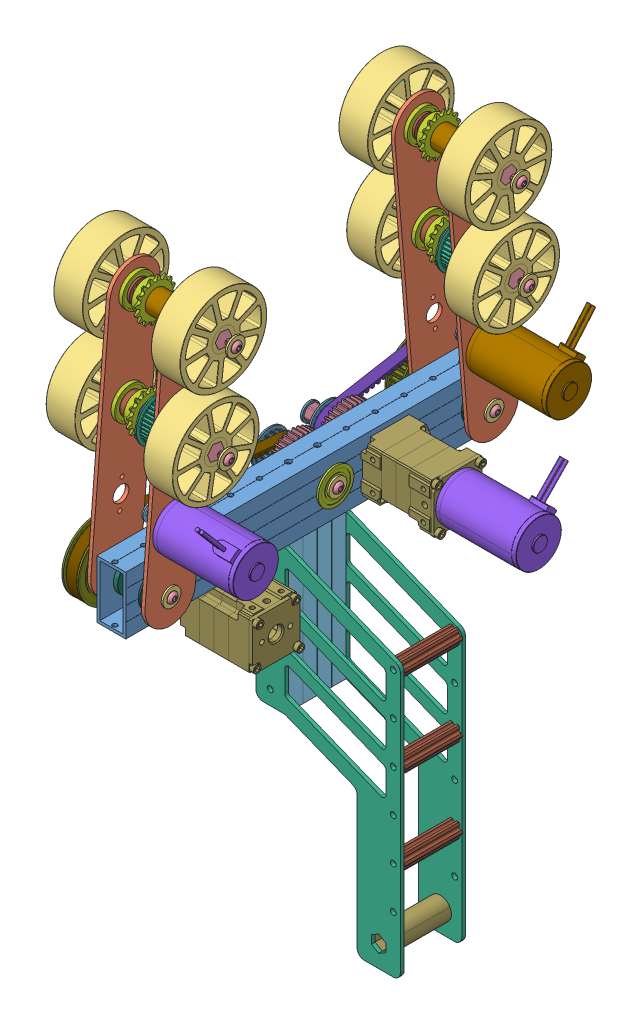
SolidWorks assembly updated grabber, configuration Default. Lengths in mm.
Overall size (217.61 560.62 367.28).
125 component instances, 32 part files, 6 mates.
Components (placement in the parent):
- 18000 - Rotational Grabber-1: 18000 - Rotational Grabber [Default] at (150.3363 402.3193 -558.2646) size (217.61 560.62 367.28)
  - 18001 - 11in Base Versaframe-1: 18001 - 11in Base Versaframe [Default] at (-59.9903 -66.9277 445.6815) size (25.4 50.8 336.55)
  - 18002 - Grabber intake plate-1: 18002 - Grabber intake plate [Default] at (-85.3649 -68.7494 1136.9284) x (0 0.081964 0.996635) z (0 0.996635 -0.081964) size (44.45 3.17 247.65)
  - 18002 - Grabber intake plate-2: 18002 - Grabber intake plate [Default] at (-85.3649 -65.1061 853.1342) x (0 -0.081964 0.996635) z (0 0.996635 0.081964) size (44.45 3.17 247.65)
  - 18002 - Grabber intake plate-3: 18002 - Grabber intake plate [Default] at (-34.6157 -68.7494 897.4346) x (0 0.081964 -0.996635) z (0 0.996635 0.081964) size (44.45 3.17 247.65)
  - 18002 - Grabber intake plate-4: 18002 - Grabber intake plate [Default] at (-34.6157 -65.1061 1181.2288) x (0 -0.081964 -0.996635) z (0 0.996635 -0.081964) size (44.45 3.17 247.65)
  - Andymark - 3in .5in Hex Compliant Wheel am-3945-1: Andymark - 3in .5in Hex Compliant Wheel am-3945 [Default] at (11.4119 85.6619 1174.5787) x (0 -0.802579 0.596545) z (-1 0 0) size (76.2 76.2 25.4)
  - Andymark - 3in .5in Hex Compliant Wheel am-3945-2: Andymark - 3in .5in Hex Compliant Wheel am-3945 [Default] at (11.4119 180.7711 930.4775) x (0 0.802579 0.596545) z (-1 0 0) size (76.2 76.2 25.4)
  - Andymark - 3in .5in Hex Compliant Wheel am-3945-3: Andymark - 3in .5in Hex Compliant Wheel am-3945 [Default] at (-74.2623 85.6619 1174.5787) x (0 -0.802579 0.596545) z (-1 0 0) size (76.2 76.2 25.4)
  - Andymark - 3in .5in Hex Compliant Wheel am-3945-4: Andymark - 3in .5in Hex Compliant Wheel am-3945 [Default] at (-131.3925 185.5152 924.0948) x (0 0.802579 0.596545) z (1 0 0) size (76.2 76.2 25.4)
  - Andymark - 3in .5in Hex Compliant Wheel am-3945-5: Andymark - 3in .5in Hex Compliant Wheel am-3945 [Default] at (-45.7183 67.5471 1206.8448) x (0 0.174088 0.98473) z (1 0 0) size (76.2 76.2 25.4)
  - Andymark - 3in .5in Hex Compliant Wheel am-3945-6: Andymark - 3in .5in Hex Compliant Wheel am-3945 [Default] at (-45.7183 59.7158 826.1337) x (0 0.174088 -0.98473) z (1 0 0) size (76.2 76.2 25.4)
  - Andymark - 3in .5in Hex Compliant Wheel am-3945-7: Andymark - 3in .5in Hex Compliant Wheel am-3945 [Default] at (-74.2623 46.9169 1090.1499) x (0 -0.174088 -0.98473) z (-1 0 0) size (76.2 76.2 25.4)
  - Andymark - 3in .5in Hex Compliant Wheel am-3945-8: Andymark - 3in .5in Hex Compliant Wheel am-3945 [Default] at (-74.2623 39.0856 942.8286) x (0 -0.174088 0.98473) z (-1 0 0) size (76.2 76.2 25.4)
  - 18003 -  Intake Shaft 4.75 in-4: 18003 -  Intake Shaft 4.75 in [Default] at (-461.6532 135.6003 1142.4147) x (0 -0.802579 0.596545) z (-1 0 0) size (14.48 12.67 120.65)
  - 18003 -  Intake Shaft 4.75 in-5: 18003 -  Intake Shaft 4.75 in [Default] at (-461.6532 53.2963 1149.2065) x (0 0.765757 -0.64313) z (-1 0 0) size (14.48 12.67 120.65)
  - 17001 - Intake Mounting Versaframe-1: 17001 - Intake Mounting Versaframe [Default] at (-59.9903 -841.6277 1017.1815) x (1 0 0) z (0 -1 0) size (25.4 50.8 127)
  - 17003 - Intake Mounting Platwe-1: 17003 - Intake Mounting Platwe [Default] at (-72.6903 -92.3277 1042.5815) x (0 -1 0) z (0 0 1) size (279.4 127 3.17)
  - 17003 - Intake Mounting Platwe-2: 17003 - Intake Mounting Platwe [Default] at (-72.6903 -92.3277 988.6065) x (0 -1 0) z (0 0 1) size (279.4 127 3.17)
  - Vexpro - .5in hex bearing flanged - 217-3875-13: Vexpro - .5in hex bearing flanged - 217-3875 [Default] at (-40.9657 53.3163 1149.1896) x (0 -0.765757 0.64313) z (0 0.64313 0.765757) size (31.12 7.94 31.12)
  - Vexpro - .5in hex bearing flanged - 217-3875-15: Vexpro - .5in hex bearing flanged - 217-3875 [Default] at (-40.9657 135.5886 1142.4234) x (0 0.917913 0.396782) z (0 0.396782 -0.917913) size (31.12 7.94 31.12)
  - Vexpro - .5in hex bearing flanged - 217-3875-16: Vexpro - .5in hex bearing flanged - 217-3875 [Default] at (-40.9657 53.3163 885.1734) x (0 -0.950153 0.311785) z (0 0.311785 0.950153) size (31.12 7.94 31.12)
  - Vexpro - .5in hex bearing flanged - 217-3875-17: Vexpro - .5in hex bearing flanged - 217-3875 [Default] at (-40.9657 135.5886 891.9395) x (0 -0.202349 0.979313) z (0 0.979313 0.202349) size (31.12 7.94 31.12)
  - Vexpro - .5in hex bearing flanged - 217-3875-19: Vexpro - .5in hex bearing flanged - 217-3875 [Default] at (-79.0149 135.5886 1142.4234) x (0 0.917913 0.396782) z (0 -0.396782 0.917913) size (31.12 7.94 31.12)
  - Vexpro - .5in hex bearing flanged - 217-3875-20: Vexpro - .5in hex bearing flanged - 217-3875 [Default] at (-79.0149 53.3163 1149.1896) x (0 -0.765757 0.64313) z (0 -0.64313 -0.765757) size (31.12 7.94 31.12)
  - Vexpro - .5in hex bearing flanged - 217-3875-21: Vexpro - .5in hex bearing flanged - 217-3875 [Default] at (-79.0149 135.5886 891.9395) x (0 -0.202349 0.979313) z (0 -0.979313 -0.202349) size (31.12 7.94 31.12)
  - Vexpro - .5in hex bearing flanged - 217-3875-22: Vexpro - .5in hex bearing flanged - 217-3875 [Default] at (-79.0149 53.3163 885.1734) x (0 -0.950153 0.311785) z (0 -0.311785 -0.950153) size (31.12 7.94 31.12)
  - Vexpro - BAG Motor - 217-3351-2: Vexpro - BAG Motor - 217-3351 [Default] at (-34.6157 -14.5013 1154.767) x (0 -0.996635 0.081964) z (-1 0 0) size (59.07 59.07 84.5)
  - 18003 -  Intake Shaft 4.75 in-6: 18003 -  Intake Shaft 4.75 in [Default] at (332.0968 53.2963 885.1565) x (0 0.765757 0.64313) z (1 0 0) size (14.48 12.67 120.65)
  - 18003 -  Intake Shaft 4.75 in-7: 18003 -  Intake Shaft 4.75 in [Default] at (332.0968 135.6003 891.9483) x (0 -0.802579 -0.596545) z (1 0 0) size (14.48 12.67 120.65)
  - MirrorVexpro - BAG Motor - 217-3351-3: MirrorVexpro - BAG Motor - 217-3351 [Default] at (-34.6157 -14.5013 879.596) x (0 -0.996635 -0.081964) z (1 0 0) size (59.07 59.07 84.5)
  - Vexpro - .125 acetal hex spacer - 217-2758-1: Vexpro - .125 acetal hex spacer - 217-2758 [Default] at (-31.4407 135.5886 891.9395) x (0 0.919668 0.392697) z (-1 0 0) size (19.05 19.05 3.17)
  - Vexpro - .125 acetal hex spacer - 217-2758-2: Vexpro - .125 acetal hex spacer - 217-2758 [Default] at (-31.4407 135.5886 1142.4234) x (0 0.919668 -0.392697) z (1 0 0) size (19.05 19.05 3.17)
  - Vexpro - .125 acetal hex spacer - 217-2758-3: Vexpro - .125 acetal hex spacer - 217-2758 [Default] at (-31.4407 53.3163 885.1734) x (0 0.919668 0.392697) z (-1 0 0) size (19.05 19.05 3.17)
  - Vexpro - .125 acetal hex spacer - 217-2758-4: Vexpro - .125 acetal hex spacer - 217-2758 [Default] at (-31.4407 53.3163 1149.1896) x (0 0.919668 -0.392697) z (1 0 0) size (19.05 19.05 3.17)
  - Vexpro - .125 acetal hex spacer - 217-2758-5: Vexpro - .125 acetal hex spacer - 217-2758 [Default] at (-88.5399 135.5886 891.9395) x (0 0.919668 0.392697) z (-1 0 0) size (19.05 19.05 3.17)
  - Vexpro - .125 acetal hex spacer - 217-2758-6: Vexpro - .125 acetal hex spacer - 217-2758 [Default] at (-88.5399 53.3163 885.1734) x (0 0.919668 0.392697) z (-1 0 0) size (19.05 19.05 3.17)
  - Vexpro - .125 acetal hex spacer - 217-2758-7: Vexpro - .125 acetal hex spacer - 217-2758 [Default] at (-88.5399 135.5886 1142.4234) x (0 0.919668 -0.392697) z (1 0 0) size (19.05 19.05 3.17)
  - Vexpro - .125 acetal hex spacer - 217-2758-8: Vexpro - .125 acetal hex spacer - 217-2758 [Default] at (-88.5399 53.3163 1149.1896) x (0 0.919668 -0.392697) z (1 0 0) size (19.05 19.05 3.17)
  - Vexpro - .25in acetal hex spacer - 217-3259-1: Vexpro - .25in acetal hex spacer - 217-3259 [Default] at (-75.8399 53.3163 885.1734) x (0 0.983572 0.180519) z (-1 0 0) size (19.5 19.5 6.35)
  - Vexpro - .25in acetal hex spacer - 217-3259-2: Vexpro - .25in acetal hex spacer - 217-3259 [Default] at (-75.8399 53.3163 1149.1896) x (0 0.983572 -0.180519) z (1 0 0) size (19.5 19.5 6.35)
  - Vexpro - .25in acetal hex spacer - 217-3259-5: Vexpro - .25in acetal hex spacer - 217-3259 [Default] at (-80.577 135.5886 891.9395) x (0 0.981987 0.188951) z (-1 0 0) size (19.5 19.5 6.35)
  - Vexpro - .25in acetal hex spacer - 217-3259-6: Vexpro - .25in acetal hex spacer - 217-3259 [Default] at (-80.577 135.5886 1142.4234) x (0 0.981987 -0.188951) z (1 0 0) size (19.5 19.5 6.35)
  - Vexpro - 100 to 1 BAG Versaplanetary Assembly-1: Vexpro - 100 to 1 BAG Versaplanetary Assembly [Default] at (-30.6653 -66.9277 934.2886) x (-1 0 0) z (0 1 0) size (107.67 44.45 42.65)
  - Vexpro - BAG Motor - 217-3351-3: Vexpro - BAG Motor - 217-3351 [Default] at (15.7347 -66.9277 956.5136) x (0 -0.014739 0.999891) z (-1 0 0) size (59.07 59.07 84.5)
  - Vexpro - 36t 20DP 0.5 Hex Gear, 217-3214-1: Vexpro - 36t 20DP 0.5 Hex Gear, 217-3214 [Default] at (-80.6024 -66.9277 956.5136) x (0 0.690037 0.723774) z (-1 0 0) size (48.16 48.16 12.65)
  - Vexpro - 36t 20DP 0.5 Hex Gear, 217-3214-2: Vexpro - 36t 20DP 0.5 Hex Gear, 217-3214 [Default] at (-80.6024 -66.9277 1002.2336) x (0 -0.981814 -0.189847) z (-1 0 0) size (48.16 48.16 12.65)
  - 18T x 9mm Wide Double Flange Aluminum Pulley (HTD 5mm, 1_2” Hex Bore) (217-3225)-1: 18T x 9mm Wide Double Flange Aluminum Pulley (HTD 5mm, 1_2” Hex Bore) (217-3225) [Default] at (-92.6149 -66.9277 956.5136) x (0 0.000638 -1) z (1 0 0) size (32 32 14.5)
  - 18T x 9mm Wide Double Flange Aluminum Pulley (HTD 5mm, 1_2” Hex Bore) (217-3225)-2: 18T x 9mm Wide Double Flange Aluminum Pulley (HTD 5mm, 1_2” Hex Bore) (217-3225) [Default] at (-97.352 -66.9277 1002.2336) x (0 0.755352 0.655319) z (-1 0 0) size (32 32 14.5)
  - Vexpro - .5in hex bearing flanged - 217-3875-27: Vexpro - .5in hex bearing flanged - 217-3875 [Default] at (-66.3403 -66.9277 956.5136) x (0 0.918835 -0.394642) z (0 0.394642 0.918835) size (31.12 7.94 31.12)
  - Vexpro - .5in hex bearing flanged - 217-3875-28: Vexpro - .5in hex bearing flanged - 217-3875 [Default] at (-66.3403 -66.9277 1002.2336) x (0 0.945199 -0.326495) z (0 0.326495 0.945199) size (31.12 7.94 31.12)
  - Vexpro - .5in hex bearing flanged - 217-3875-29: Vexpro - .5in hex bearing flanged - 217-3875 [Default] at (-53.6403 -66.9277 1002.2336) x (0 0.945199 -0.326495) z (0 -0.326495 -0.945199) size (31.12 7.94 31.12)
  - Vexpro - 13.75mm Thunderhex Bearing - 217-4006-1: Vexpro - 13.75mm Thunderhex Bearing - 217-4006 [Default] at (-49.6715 -66.9277 1159.0786) x (0 -0.259596 -0.965717) z (1 0 0) size (31.12 31.12 7.94)
  - Vexpro - 13.75mm Thunderhex Bearing - 217-4006-4: Vexpro - 13.75mm Thunderhex Bearing - 217-4006 [Default] at (-70.309 -66.9277 1159.0786) x (0 0.259596 0.965717) z (-1 0 0) size (31.12 31.12 7.94)
  - Vexpro - 13.75mm Thunderhex Bearing - 217-4006-3: Vexpro - 13.75mm Thunderhex Bearing - 217-4006 [Default] at (-49.6715 -66.9277 875.2844) x (0 0.259596 -0.965717) z (1 0 0) size (31.12 31.12 7.94)
  - Vexpro - 13.75mm Thunderhex Bearing - 217-4006-5: Vexpro - 13.75mm Thunderhex Bearing - 217-4006 [Default] at (-70.309 -66.9277 875.2844) x (0 -0.259596 0.965717) z (-1 0 0) size (31.12 31.12 7.94)
  - 36t Pulley HTD5-1: 36t Pulley HTD5 [Default] at (-92.6149 -66.9277 875.2844) x (0 -0.569301 0.822129) z (-1 0 0) size (60 60 14.5)
  - 60t Belt-2: 60t Belt [Default] at (-91.6149 -66.9277 915.899) x (0 0 -1) z (0 -1 0) size (126.54 9 59.64)
  - 90t Belt (1)-2: 90t Belt (1) [Default] at (-91.6149 -66.9277 1080.6561) x (0 0 1) z (0 1 0) size (202.16 9 59.64)
  - 36t Pulley HTD5-3: 36t Pulley HTD5 [Default] at (-92.6149 -66.9277 1159.0786) x (0 -0.569301 -0.822129) z (1 0 0) size (60 60 14.5)
  - 18004 - Intake Rotation Shaft-1: 18004 - Intake Rotation Shaft [Default] at (-491.8157 -66.6646 875.306) x (0 0.996635 0.081964) z (-1 0 0) size (13.74 12.75 74.93)
  - 18004 - Intake Rotation Shaft-2: 18004 - Intake Rotation Shaft [Default] at (347.6543 -66.6646 1159.057) x (0 0.996635 -0.081964) z (1 0 0) size (13.74 12.75 74.93)
  - Gear shaft 2-1: Gear shaft 2 [Default] at (-502.874 -66.9277 1002.2336) x (0 0.945199 -0.326495) z (-1 0 0) size (13.74 12.75 58.93)
  - McMaster - .25 ID washer - 96765A140-6: McMaster - .25 ID washer - 96765A140 [96765A140] at (-106.126 -66.9277 1002.2336) x (0 -0.992326 0.123647) z (0 0.123647 0.992326) size (15.88 1.52 15.88)
  - McMaster - .25 ID washer - 96765A140-7: McMaster - .25 ID washer - 96765A140 [96765A140] at (-45.7028 -66.9277 1002.2336) x (0 0.885672 -0.464312) z (0 -0.464312 -0.885672) size (15.88 1.52 15.88)
  - McMaster - 10-32 .3125in button head screw - 97763A706-7: McMaster - 10-32 .3125in button head screw - 97763A706 [97763A706] at (-103.4399 -66.9277 1002.2336) x (0 0.999782 0.020866) z (-1 0 0) size (9.17 9.17 10.95)
  - McMaster - 10-32 .3125in button head screw - 97763A706-8: McMaster - 10-32 .3125in button head screw - 97763A706 [97763A706] at (-46.8648 -66.9277 1002.2336) x (0 0.489689 -0.871897) z (1 0 0) size (9.17 9.17 10.95)
  - McMaster - 10-32 .3125in button head screw - 97763A706-9: McMaster - 10-32 .3125in button head screw - 97763A706 [97763A706] at (-47.1442 -84.8882 974.4741) x (0 0.999782 0.020866) z (-1 0 0) size (9.17 9.17 10.95)
  - McMaster - 10-32 .3125in button head screw - 97763A706-10: McMaster - 10-32 .3125in button head screw - 97763A706 [97763A706] at (-47.1442 -48.9672 938.5531) x (0 0.990973 0.134063) z (-1 0 0) size (9.17 9.17 10.95)
  - Vexpro - BAG 12T GT2 9mm - 217-5872-1: Vexpro - BAG 12T GT2 9mm - 217-5872 [Default] at (-48.0907 -14.5013 1154.767) x (0 0.214456 0.976734) z (1 0 0) size (15 15 17.5)
  - Vexpro - 36T GT2 9mm Wide - 217-5873-1: Vexpro - 36T GT2 9mm Wide - 217-5873 [Default] at (-48.9032 53.3163 1149.1896) x (0 0.207951 0.978139) z (-1 0 0) size (39 39 15.88)
  - Vexpro - 16t .5 in Hex Hub Sprocket - 217-2642-1: Vexpro - 16t .5 in Hex Hub Sprocket - 217-2642 [Default] at (-66.2831 53.3163 1149.1896) x (0 0 -1) z (1 0 0) size (35.22 35.22 9.18)
  - Vexpro - .5in acetal hex spacer - 217 - 3261-1: Vexpro - .5in acetal hex spacer - 217 - 3261 [Default] at (-57.1391 53.3163 1149.1896) x (0 0.125259 -0.992124) z (1 0 0) size (19.5 19.5 12.7)
  - Vexpro - 16t .5 in Hex Hub Sprocket - 217-2642-2: Vexpro - 16t .5 in Hex Hub Sprocket - 217-2642 [Default] at (-66.2831 135.5886 1142.4234) x (0 0.415394 -0.909641) z (1 0 0) size (35.22 35.22 9.18)
  - Vexpro - .125 acetal hex spacer - 217-2758-13: Vexpro - .125 acetal hex spacer - 217-2758 [Default] at (-88.5145 -66.9277 1002.2336) x (0 0.919668 0.392697) z (-1 0 0) size (19.05 19.05 3.17)
  - Vexpro - .5in acetal hex spacer - 217 - 3261-2: Vexpro - .5in acetal hex spacer - 217 - 3261 [Default] at (-75.8399 -66.9277 875.2844) x (0 -0.683534 -0.729919) z (-1 0 0) size (19.5 19.5 12.7)
  - Vexpro - .125 acetal hex spacer - 217-2758-14: Vexpro - .125 acetal hex spacer - 217-2758 [Default] at (-49.2016 53.3163 1149.1896) x (0 0.919029 0.39419) z (1 0 0) size (19.05 19.05 3.17)
  - Vexpro - 1in acetal hex spacer - 217-3263-6: Vexpro - 1in acetal hex spacer - 217-3263 [Default] at (-50.7891 135.5886 1142.4234) x (0 0.039594 -0.999216) z (1 0 0) size (19.5 19.5 25.4)
  - Vexpro - .25in acetal hex spacer - 217-3259-7: Vexpro - .25in acetal hex spacer - 217-3259 [Default] at (-34.9141 135.5886 1142.4234) x (0 0.023558 -0.999722) z (1 0 0) size (19.5 19.5 6.35)
  - Vexpro - 16t .5 in Hex Hub Sprocket - 217-2642-5: Vexpro - 16t .5 in Hex Hub Sprocket - 217-2642 [Default] at (-66.2831 135.5886 891.9395) x (0 0.415394 0.909641) z (1 0 0) size (35.22 35.22 9.18)
  - Vexpro - 1in acetal hex spacer - 217-3263-7: Vexpro - 1in acetal hex spacer - 217-3263 [Default] at (-50.7891 135.5886 891.9395) x (0 0.039594 0.999216) z (-1 0 0) size (19.5 19.5 25.4)
  - Vexpro - .25in acetal hex spacer - 217-3259-8: Vexpro - .25in acetal hex spacer - 217-3259 [Default] at (-34.9141 135.5886 891.9395) x (0 0.023558 0.999722) z (-1 0 0) size (19.5 19.5 6.35)
  - Vexpro - 16t .5 in Hex Hub Sprocket - 217-2642-6: Vexpro - 16t .5 in Hex Hub Sprocket - 217-2642 [Default] at (-66.2831 53.3163 885.1734) x (0 0 1) z (1 0 0) size (35.22 35.22 9.18)
  - Vexpro - .5in acetal hex spacer - 217 - 3261-5: Vexpro - .5in acetal hex spacer - 217 - 3261 [Default] at (-57.1391 53.3163 885.1734) x (0 0.125259 0.992124) z (-1 0 0) size (19.5 19.5 12.7)
  - Vexpro - .125 acetal hex spacer - 217-2758-18: Vexpro - .125 acetal hex spacer - 217-2758 [Default] at (-49.2016 53.3163 885.1734) x (0 0.919029 -0.39419) z (-1 0 0) size (19.05 19.05 3.17)
  - Vexpro - 36T GT2 9mm Wide - 217-5873-4: Vexpro - 36T GT2 9mm Wide - 217-5873 [Default] at (-48.9032 53.3163 885.1734) x (0 0.207951 -0.978139) z (1 0 0) size (39 39 15.88)
  - Vexpro - .5in acetal hex spacer - 217 - 3261-6: Vexpro - .5in acetal hex spacer - 217 - 3261 [Default] at (-75.8399 -66.9277 1159.0786) x (0 -0.683534 0.729919) z (1 0 0) size (19.5 19.5 12.7)
  - Vexpro - .5in acetal hex spacer - 217 - 3261-7: Vexpro - .5in acetal hex spacer - 217 - 3261 [Default] at (-44.1407 -66.9277 1159.0786) x (0 -0.683534 0.729919) z (1 0 0) size (19.5 19.5 12.7)
  - Vexpro - .5in acetal hex spacer - 217 - 3261-8: Vexpro - .5in acetal hex spacer - 217 - 3261 [Default] at (-44.1407 -66.9277 875.2844) x (0 -0.683534 -0.729919) z (-1 0 0) size (19.5 19.5 12.7)
  - Vexpro - BAG 12T GT2 9mm - 217-5872-2: Vexpro - BAG 12T GT2 9mm - 217-5872 [Default] at (-48.0907 -14.5013 879.596) x (0 0.214456 -0.976734) z (-1 0 0) size (15 15 17.5)
  - Vexpro - 100 to 1 BAG Versaplanetary Assembly-2: Vexpro - 100 to 1 BAG Versaplanetary Assembly [Default] at (-53.6403 -136.7777 1093.3815) x (-1 0 0) z (0 0 -1) size (107.67 44.45 42.65)
  - McMaster - .25 ID washer - 96765A140-8: McMaster - .25 ID washer - 96765A140 [96765A140] at (-111.0697 -66.9277 1159.0786) x (0 -0.999378 -0.035253) z (0 -0.035253 0.999378) size (15.88 1.52 15.88)
  - McMaster - 10-32 .3125in button head screw - 97763A706-11: McMaster - 10-32 .3125in button head screw - 97763A706 [97763A706] at (-108.3836 -66.9277 1159.0786) x (0 0.983827 0.179121) z (-1 0 0) size (9.17 9.17 10.95)
  - McMaster - .25 ID washer - 96765A140-10: McMaster - .25 ID washer - 96765A140 [96765A140] at (-126.6272 53.3163 1149.1896) x (0 -0.815677 -0.578508) z (0 -0.578508 0.815677) size (15.88 1.52 15.88)
  - McMaster - 10-32 .3125in button head screw - 97763A706-13: McMaster - 10-32 .3125in button head screw - 97763A706 [97763A706] at (-123.9411 53.3163 1149.1896) x (0 0.723643 0.690174) z (-1 0 0) size (9.17 9.17 10.95)
  - McMaster - .25 ID washer - 96765A140-12: McMaster - .25 ID washer - 96765A140 [96765A140] at (-126.6272 135.5886 1142.4234) x (0 -0.702828 -0.71136) z (0 -0.71136 0.702828) size (15.88 1.52 15.88)
  - McMaster - 10-32 .3125in button head screw - 97763A706-15: McMaster - 10-32 .3125in button head screw - 97763A706 [97763A706] at (-123.9411 135.5886 1142.4234) x (0 0.840015 -0.542564) z (-1 0 0) size (9.17 9.17 10.95)
  - McMaster - 10-32 .3125in button head screw - 97763A706-17: McMaster - 10-32 .3125in button head screw - 97763A706 [97763A706] at (-123.9411 135.5886 891.9395) x (0 -0.840015 -0.542564) z (-1 0 0) size (9.17 9.17 10.95)
  - McMaster - .25 ID washer - 96765A140-14: McMaster - .25 ID washer - 96765A140 [96765A140] at (-126.6272 135.5886 891.9395) x (0 -0.702828 0.71136) z (0 0.71136 0.702828) size (15.88 1.52 15.88)
  - McMaster - 10-32 .3125in button head screw - 97763A706-18: McMaster - 10-32 .3125in button head screw - 97763A706 [97763A706] at (-123.9411 53.3163 885.1734) x (0 -0.723643 0.690174) z (-1 0 0) size (9.17 9.17 10.95)
  - McMaster - .25 ID washer - 96765A140-15: McMaster - .25 ID washer - 96765A140 [96765A140] at (-126.6272 53.3163 885.1734) x (0 -0.815677 0.578508) z (0 0.578508 0.815677) size (15.88 1.52 15.88)
  - McMaster - 10-32 .3125in button head screw - 97763A706-19: McMaster - 10-32 .3125in button head screw - 97763A706 [97763A706] at (-108.3836 -66.9277 875.2844) x (0 -0.983827 0.179121) z (-1 0 0) size (9.17 9.17 10.95)
  - McMaster - .25 ID washer - 96765A140-16: McMaster - .25 ID washer - 96765A140 [96765A140] at (-111.0697 -66.9277 875.2844) x (0 -0.999378 0.035253) z (0 0.035253 0.999378) size (15.88 1.52 15.88)
  - McMaster - 10-32 .3125in button head screw - 97763A706-20: McMaster - 10-32 .3125in button head screw - 97763A706 [97763A706] at (3.9606 53.3163 1149.1896) x (0 -0.723643 -0.690174) z (1 0 0) size (9.17 9.17 10.95)
  - McMaster - .25 ID washer - 96765A140-17: McMaster - .25 ID washer - 96765A140 [96765A140] at (6.6466 53.3163 1149.1896) x (0 -0.815677 -0.578508) z (0 0.578508 -0.815677) size (15.88 1.52 15.88)
  - McMaster - 10-32 .3125in button head screw - 97763A706-22: McMaster - 10-32 .3125in button head screw - 97763A706 [97763A706] at (3.9606 135.5886 1142.4234) x (0 -0.840015 0.542564) z (1 0 0) size (9.17 9.17 10.95)
  - McMaster - .25 ID washer - 96765A140-19: McMaster - .25 ID washer - 96765A140 [96765A140] at (6.6466 135.5886 1142.4234) x (0 -0.702828 -0.71136) z (0 0.71136 -0.702828) size (15.88 1.52 15.88)
  - McMaster - 10-32 .3125in button head screw - 97763A706-23: McMaster - 10-32 .3125in button head screw - 97763A706 [97763A706] at (3.9606 135.5886 891.9395) x (0 0.840015 0.542564) z (1 0 0) size (9.17 9.17 10.95)
  - McMaster - .25 ID washer - 96765A140-20: McMaster - .25 ID washer - 96765A140 [96765A140] at (6.6466 135.5886 891.9395) x (0 -0.702828 0.71136) z (0 -0.71136 -0.702828) size (15.88 1.52 15.88)
  - McMaster - 10-32 .3125in button head screw - 97763A706-24: McMaster - 10-32 .3125in button head screw - 97763A706 [97763A706] at (3.9606 53.3163 885.1734) x (0 0.723643 -0.690174) z (1 0 0) size (9.17 9.17 10.95)
  - McMaster - .25 ID washer - 96765A140-21: McMaster - .25 ID washer - 96765A140 [96765A140] at (6.6466 53.3163 885.1734) x (0 -0.815677 0.578508) z (0 -0.578508 -0.815677) size (15.88 1.52 15.88)
  - McMaster - .25 ID washer - 96765A140-23: McMaster - .25 ID washer - 96765A140 [96765A140] at (-33.0917 -66.6646 1159.057) x (0 -0.19415 -0.980972) z (0 0.980972 -0.19415) size (15.88 1.52 15.88)
  - McMaster - 10-32 .3125in button head screw - 97763A706-26: McMaster - 10-32 .3125in button head screw - 97763A706 [97763A706] at (-35.7777 -66.6646 1159.057) x (0 0.347239 0.937777) z (1 0 0) size (9.17 9.17 10.95)
  - McMaster - .25 ID washer - 96765A140-25: McMaster - .25 ID washer - 96765A140 [96765A140] at (-33.0917 -66.6646 875.306) x (0 -0.19415 0.980972) z (0 -0.980972 -0.19415) size (15.88 1.52 15.88)
  - McMaster - 10-32 .3125in button head screw - 97763A706-28: McMaster - 10-32 .3125in button head screw - 97763A706 [97763A706] at (-35.7777 -66.6646 875.306) x (0 -0.347239 0.937777) z (1 0 0) size (9.17 9.17 10.95)
  - 2x1x.1in Block-1: 2x1x.1in Block [Default] at (-59.9903 -105.0277 1017.1815) x (1 0 0) z (0 -1 0) size (19.05 44.45 25.4)
  - 2in churro-1: 2in churro [Default] at (47.9597 -138.0477 991.7815) size (14.66 12.7 50.8)
  - 2in churro-2: 2in churro [Default] at (47.9597 -211.7077 991.7815) size (14.66 12.7 50.8)
  - 2in churro-3: 2in churro [Default] at (47.9597 -285.3677 991.7815) size (14.66 12.7 50.8)
  - Vexpro - 2in acetal hex spacer217-3265-1: Vexpro - 2in acetal hex spacer217-3265 [Default] at (35.3867 -352.4577 1017.1815) x (0.866025 0.5 0) z (0 0 1) size (19.5 19.5 50.8)
- Threaded Hex Standoff 1 in-1: Threaded Hex Standoff 1 in [93505A197] at (62.4708 335.3916 398.249) x (0 -0.500868 0.865524) z (-1 0 0) size (12.7 14.27 38.8)
- McMaster - 10-32 .3125in button head screw - 97763A706-1: McMaster - 10-32 .3125in button head screw - 97763A706 [97763A706] at (38.2329 335.3916 398.249) x (0 -0.810726 -0.585426) z (-1 0 0) size (9.17 9.17 10.95)
- McMaster - .25 ID washer - 96765A140-1: McMaster - .25 ID washer - 96765A140 [96765A140] at (44.2103 335.3916 443.969) x (0 -0.992326 0.123647) z (0 0.123647 0.992326) size (15.88 1.52 15.88)
- McMaster - .25 ID washer - 96765A140-3: McMaster - .25 ID washer - 96765A140 [96765A140] at (44.2103 335.3916 443.969) x (0 -0.992326 0.123647) z (0 0.123647 0.992326) size (15.88 1.52 15.88)
- .25 washer-1: .25 washer [96765A140] at (37.0708 335.3916 398.249) x (0 1 0) z (0 0 1) size (15.88 1.52 15.88)
Mates (geometry in assembly coordinates):
- Concentric11: concentric anti-aligned: circle of 18000 - Rotational Grabber-1/Vexpro - 100 to 1 BAG Versaplanetary Assembly-1; circle of Threaded Hex Standoff 1 in-1
- Coincident12: coincident anti-aligned: plane of 18000 - Rotational Grabber-1/Vexpro - 100 to 1 BAG Versaplanetary Assembly-1 through (62.4708 339.0577 404.599) normal (-1 0 0); plane of Threaded Hex Standoff 1 in-1 through (62.4708 337.7005 399.5851) normal (1 0 0)
- Coincident15: coincident anti-aligned: plane of Threaded Hex Standoff 1 in-1 through (37.0708 338.4144 399.9983) normal (-1 0 0); plane of .25 washer-1 through (37.0708 335.3916 398.249) normal (1 0 0)
- Concentric16: concentric aligned: circle of Threaded Hex Standoff 1 in-1; circle of .25 washer-1
- Concentric17: concentric aligned: circle of McMaster - 10-32 .3125in button head screw - 97763A706-1; circle of .25 washer-1
- Coincident16: coincident anti-aligned: plane of McMaster - 10-32 .3125in button head screw - 97763A706-1 through (35.5468 332.7076 401.966) normal (1 0 0); plane of .25 washer-1 through (35.5468 335.3916 398.249) normal (-1 0 0)
